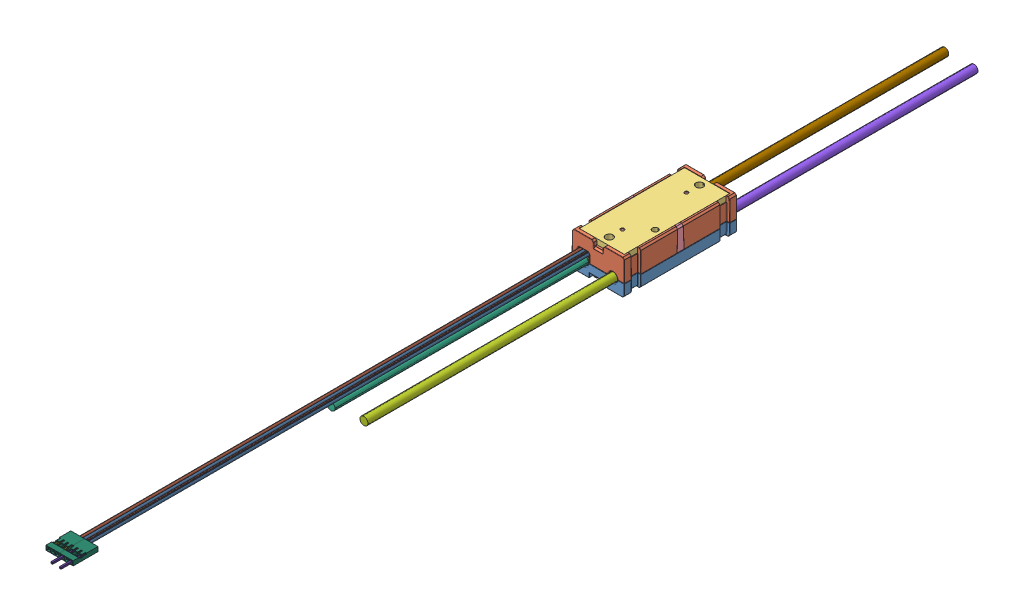
SolidWorks assembly Victor SPX (217-9191), configuration Default. Lengths in mm.
Overall size (30.33 19.59 504.96).
28 component instances, 17 part files, 0 mates.
Components (placement in the parent):
- Victor SPX (217-9191).step-1: Victor SPX (217-9191).step [Default] at origin size (30.33 19.59 504.96)
  - 217-9191-001 Rev3.step-1: 217-9191-001 Rev3.step [Default] at origin size (29.5 7.14 63.51)
  - 217-9191-002 Rev3.step-1: 217-9191-002 Rev3.step [Default] at (0 2.7 0) size (29.5 14.95 63.52)
  - 217-9191-003 Rev1.step-1: 217-9191-003 Rev1.step [Default] at (0 9.35 0) size (25.3 3 59.3)
  - 217-9191-004 Rev2.step-1: 217-9191-004 Rev2.step [Default] at (6.795 4.495 0.0018) size (4.25 13.1 6.9)
  - 217-9191-004 Rev2.step-2: 217-9191-004 Rev2.step [Default] at (-6.795 4.495 0.0018) x (-1 0 0) z (0 0 -1) size (4.25 13.1 6.9)
  - 217-9191-006 Rev2.step-1: 217-9191-006 Rev2.step [Default] at (9.2964 8.362 8.8672) x (0 0 -1) z (1 0 0) size (6.09 10.55 6.09)
  - 217-9191-911 Rev1_RED.step-1: 217-9191-911 Rev1_RED.step [Default] at (-8.25 0 21.5739) x (0.999994 0.00336 0) z (0 0 1) size (4.5 4.5 156.4)
  - 217-9191-912 Rev1_Black.step-1: 217-9191-912 Rev1_Black.step [Default] at (8.25 0 19.558) x (0.697815 -0.716278 0) z (0 0 1) size (4.5 4.5 156.4)
  - 217-9191-913 Rev1_White.step-1: 217-9191-913 Rev1_White.step [Default] at (8.25 0 -19.431) x (-0.549241 0.835664 0) z (0 0 -1) size (4.5 4.5 156.4)
  - 217-9191-914 Rev1_Black.step-1: 217-9191-914 Rev1_Black.step [Default] at (-8.25 0 -19.431) x (-0.472775 0.881183 0) z (0 0 -1) size (4.5 4.5 156.4)
  - 217-9191-915 Rev1.step-1: 217-9191-915 Rev1.step [Default] at (-7.1946 -1.0626 7.493) x (0.370352 -0.928891 0) z (0 0 -1) size (6.7 1.5 308.78)
  - 217-9191-916 Rev1.step-1: 217-9191-916 Rev1.step [Default] at (-9.2392 -1.0626 7.493) x (-0.369925 -0.929062 0) z (0 0 -1) size (6.7 1.5 308.78)
  - 217-9191-915 Rev1.step-2: 217-9191-915 Rev1.step [Default] at (-6.3946 -1.0626 7.493) x (-0.103805 -0.994598 0) z (0 0 -1) size (6.7 1.5 308.78)
  - 217-9191-916 Rev1.step-2: 217-9191-916 Rev1.step [Default] at (-10.0392 -1.0626 7.493) x (0.104202 -0.994556 0) z (0 0 -1) size (6.7 1.5 308.78)
  - 217-9191-005 Rev1.step-1: 217-9191-005 Rev1.step [Default] at (-8.25 0 26.133) size (7.74 4.36 11.03)
  - 217-9191-007 Rev1_92005A071.step-1: 217-9191-007 Rev1_92005A071.step [Default] at (0 12.05 18) x (-0.856814 0 0.515625) z (0 -1 0) size (5 5 6.64)
  - 217-9191-007 Rev1_92005A071.step-2: 217-9191-007 Rev1_92005A071.step [Default] at (0 12.05 -18) x (1 0 0) z (0 -1 0) size (5 5 6.64)
  - 217-9191-008 Rev1.step-1: 217-9191-008 Rev1.step [Default] at (-78.6347 -3.05 22.1716) x (0.778462 0 -0.627691) z (0 -1 0) size (4.2 4.2 11.81)
  - 217-9191-008 Rev1.step-2: 217-9191-008 Rev1.step [Default] at (15.0561 -3.05 -46.2819) x (0.568576 0 0.822631) z (0 -1 0) size (4.2 4.2 11.81)
  - 217-9191-008 Rev1.step-3: 217-9191-008 Rev1.step [Default] at (-52.1 -3.05 -81.77) x (1 0 0) z (0 -1 0) size (4.2 4.2 11.81)
  - 217-9191-008 Rev1.step-4: 217-9191-008 Rev1.step [Default] at (-57.6 -3.05 -81.77) x (1 0 0) z (0 -1 0) size (4.2 4.2 11.81)
  - 217-9090-018 Rev1.step-1: 217-9090-018 Rev1.step [Default] at (-11.7479 3.8841 320.2778) size (7.66 2.5 14)
  - 217-9090-019 Rev1.step-1: 217-9090-019 Rev1.step [Default] at (-14.3254 4.0591 320.2778) size (1.6 1.6 12)
  - 217-9090-019 Rev1.step-2: 217-9090-019 Rev1.step [Default] at (-9.1704 4.0591 320.2778) size (1.6 1.6 12)
  - 217-9090-018 Rev1.step-2: 217-9090-018 Rev1.step [Default] at (-4.0879 3.8841 320.2778) size (7.66 2.5 14)
  - 217-9191-017 Rev1.step-1: 217-9191-017 Rev1.step [Default] at (-6.4904 3.8841 320.2778) size (1.6 1.6 18.85)
  - 217-9191-017 Rev1.step-2: 217-9191-017 Rev1.step [Default] at (-1.6854 3.8841 320.2778) size (1.6 1.6 18.85)
